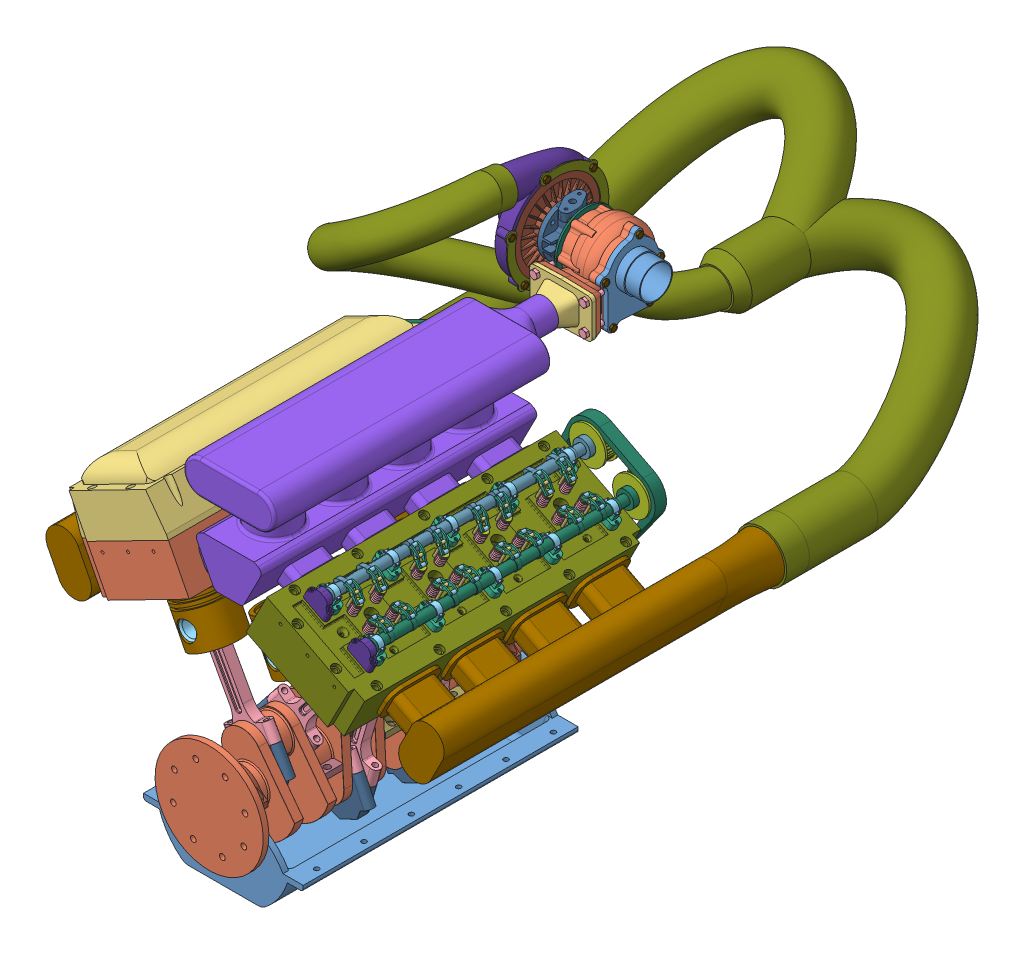
SolidWorks assembly ENSAMBLAJE DE MOTOR V8, configuration Predeterminado. Lengths in mm. (continued)
Mates (geometry in assembly coordinates): (continued)
- Concéntrica259: concentric: cylinder of CUBIERTA DE SOPORTE DE ARBOL DE LEVAS-22 through (209.4015 209.8469 383.5) axis (0.455744 0.890111 0) radius 1.25; cylinder of SOPORTE DE ARBOL DE LEVAS-22 through (208.0343 207.1766 383.5) axis (0.455744 0.890111 0) radius 1
- Concéntrica260: concentric: cylinder of CUBIERTA DE SOPORTE DE ARBOL DE LEVAS-22 through (209.4015 209.8469 389.5) axis (0.455744 0.890111 0) radius 1.25; cylinder of SOPORTE DE ARBOL DE LEVAS-22 through (208.0343 207.1766 389.5) axis (0.455744 0.890111 0) radius 1
- Concéntrica261: concentric: cylinder of assembly; cylinder of assembly; cylinder of CUBIERTA DE SOPORTE DE ARBOL DE LEVAS-23 through (121.6935 251.3837 391.5) axis (0 0 -1) radius 9.9624; cylinder of SOPORTE DE ARBOL DE LEVAS-23 through (121.6935 251.3837 391.5) axis (0 0 -1) radius 8.5
- Concéntrica262: concentric: cylinder of CUBIERTA DE SOPORTE DE ARBOL DE LEVAS-23 through (132.8519 249.0408 389.5) axis (0.455744 0.890111 0) radius 1.25; cylinder of SOPORTE DE ARBOL DE LEVAS-23 through (131.4847 246.3705 389.5) axis (0.455744 0.890111 0) radius 1
- Concéntrica263: concentric: cylinder of CUBIERTA DE SOPORTE DE ARBOL DE LEVAS-23 through (132.8519 249.0408 383.5) axis (0.455744 0.890111 0) radius 1.25; cylinder of SOPORTE DE ARBOL DE LEVAS-23 through (131.4847 246.3705 383.5) axis (0.455744 0.890111 0) radius 1
- Concéntrica264: concentric: cylinder of assembly; cylinder of assembly; cylinder of CUBIERTA DE SOPORTE DE ARBOL DE LEVAS-21 through (198.243 212.1897 288.5) axis (0 0 -1) radius 9.9624; cylinder of SOPORTE DE ARBOL DE LEVAS-21 through (198.243 212.1897 288.5) axis (0 0 -1) radius 8.5
- Concéntrica265: concentric: cylinder of CUBIERTA DE SOPORTE DE ARBOL DE LEVAS-21 through (209.4015 209.8469 286.5) axis (0.455744 0.890111 0) radius 1.25; cylinder of SOPORTE DE ARBOL DE LEVAS-21 through (208.0343 207.1766 286.5) axis (0.455744 0.890111 0) radius 1
- Concéntrica266: concentric: cylinder of CUBIERTA DE SOPORTE DE ARBOL DE LEVAS-21 through (209.4015 209.8469 280.5) axis (0.455744 0.890111 0) radius 1; cylinder of SOPORTE DE ARBOL DE LEVAS-21 through (208.0343 207.1766 280.5) axis (0.455744 0.890111 0) radius 1
- Paralelo12: parallel: cylinder of CUBIERTA DE SOPORTE DE ARBOL DE LEVAS-18 through (209.4015 209.8469 492.5) axis (0.455744 0.890111 0) radius 1.25; cylinder of SOPORTE DE ARBOL DE LEVAS-18 through (208.8175 195.541 489.5) axis (0.455744 0.890111 0) radius 2.5
- Concéntrica268: concentric: cylinder of CUBIERTA DE SOPORTE DE ARBOL DE LEVAS-18 through (209.4015 209.8469 486.5) axis (0.455744 0.890111 0) radius 1.25; circle of SOPORTE DE ARBOL DE LEVAS-18
- Concéntrica269: concentric: cylinder of CUBIERTA DE SOPORTE DE ARBOL DE LEVAS-18 through (198.243 212.1897 494.5) axis (0 0 -1) radius 9.9624; cylinder of SOPORTE DE ARBOL DE LEVAS-18 through (198.243 212.1897 494.5) axis (0 0 -1) radius 8.5
- Concéntrica270: concentric: cylinder of assembly; cylinder of assembly; cylinder of CUBIERTA DE SOPORTE DE ARBOL DE LEVAS-16 through (198.243 212.1897 597.5) axis (0 0 -1) radius 9.9624; cylinder of SOPORTE DE ARBOL DE LEVAS-16 through (198.243 212.1897 597.5) axis (0 0 -1) radius 8.5
- Concéntrica271: concentric: cylinder of CUBIERTA DE SOPORTE DE ARBOL DE LEVAS-16 through (189.8191 219.8733 595.5) axis (0.455744 0.890111 0) radius 1; cylinder of SOPORTE DE ARBOL DE LEVAS-16 through (188.4518 217.2029 595.5) axis (0.455744 0.890111 0) radius 1
- Concéntrica272: concentric: cylinder of CUBIERTA DE SOPORTE DE ARBOL DE LEVAS-16 through (189.8191 219.8733 589.5) axis (0.455744 0.890111 0) radius 1.25; cylinder of SOPORTE DE ARBOL DE LEVAS-16 through (188.4518 217.2029 589.5) axis (0.455744 0.890111 0) radius 1
- Concéntrica274: concentric: cylinder of assembly; cylinder of assembly; cylinder of CUBIERTA DE SOPORTE DE ARBOL DE LEVAS-20 through (121.6935 251.3837 597.5) axis (0 0 -1) radius 9.9624; cylinder of SOPORTE DE ARBOL DE LEVAS-20 through (121.6935 251.3837 597.5) axis (0 0 -1) radius 8.5
- Concéntrica275: concentric: cylinder of CUBIERTA DE SOPORTE DE ARBOL DE LEVAS-20 through (113.2695 259.0672 595.5) axis (0.455744 0.890111 0) radius 1.25; cylinder of SOPORTE DE ARBOL DE LEVAS-20 through (111.9023 256.3969 595.5) axis (0.455744 0.890111 0) radius 1
- Concéntrica276: concentric: cylinder of CUBIERTA DE SOPORTE DE ARBOL DE LEVAS-20 through (113.2695 259.0672 589.5) axis (0.455744 0.890111 0) radius 1.25; cylinder of SOPORTE DE ARBOL DE LEVAS-20 through (111.9023 256.3969 589.5) axis (0.455744 0.890111 0) radius 1
- Concéntrica277: concentric: cylinder of assembly; cylinder of assembly; cylinder of CUBIERTA DE SOPORTE DE ARBOL DE LEVAS-19 through (121.6935 251.3837 494.5) axis (0 0 -1) radius 9.9624; cylinder of SOPORTE DE ARBOL DE LEVAS-19 through (121.6935 251.3837 494.5) axis (0 0 -1) radius 8.5
- Concéntrica278: concentric: cylinder of CUBIERTA DE SOPORTE DE ARBOL DE LEVAS-19 through (113.2695 259.0672 492.5) axis (0.455744 0.890111 0) radius 1; cylinder of SOPORTE DE ARBOL DE LEVAS-19 through (111.9023 256.3969 492.5) axis (0.455744 0.890111 0) radius 1
- Concéntrica279: concentric: cylinder of CUBIERTA DE SOPORTE DE ARBOL DE LEVAS-19 through (113.2695 259.0672 486.5) axis (0.455744 0.890111 0) radius 1.25; cylinder of SOPORTE DE ARBOL DE LEVAS-19 through (111.9023 256.3969 486.5) axis (0.455744 0.890111 0) radius 1
- Concéntrica280: concentric: cylinder of assembly; cylinder of assembly; cylinder of CUBIERTA DE SOPORTE DE ARBOL DE LEVAS-15 through (-150.1483 251.4202 408.25) axis (0 0 -1) radius 9.9624; cylinder of SOPORTE DE ARBOL DE LEVAS-15 through (-150.1483 251.4202 408.25) axis (0 0 -1) radius 8.5
- Concéntrica281: concentric: cylinder of CUBIERTA DE SOPORTE DE ARBOL DE LEVAS-15 through (-161.3067 249.0773 400.25) axis (-0.455744 0.890111 0) radius 1; cylinder of SOPORTE DE ARBOL DE LEVAS-15 through (-159.9395 246.407 400.25) axis (-0.455744 0.890111 0) radius 1
- Concéntrica282: concentric: cylinder of CUBIERTA DE SOPORTE DE ARBOL DE LEVAS-15 through (-161.3067 249.0773 406.25) axis (-0.455744 0.890111 0) radius 1.25; cylinder of SOPORTE DE ARBOL DE LEVAS-15 through (-159.9395 246.407 406.25) axis (-0.455744 0.890111 0) radius 1
- Concéntrica283: concentric: cylinder of assembly; cylinder of assembly; cylinder of CUBIERTA DE SOPORTE DE ARBOL DE LEVAS-17 through (121.6935 251.3837 700.5) axis (0 0 -1) radius 9.9624; cylinder of SOPORTE DE ARBOL DE LEVAS-17 through (121.6935 251.3837 700.5) axis (0 0 -1) radius 8.5
- Concéntrica284: concentric: cylinder of CUBIERTA DE SOPORTE DE ARBOL DE LEVAS-17 through (113.2695 259.0672 698.5) axis (0.455744 0.890111 0) radius 1; cylinder of SOPORTE DE ARBOL DE LEVAS-17 through (111.9023 256.3969 698.5) axis (0.455744 0.890111 0) radius 1
- Concéntrica285: concentric: cylinder of CUBIERTA DE SOPORTE DE ARBOL DE LEVAS-17 through (113.2695 259.0672 692.5) axis (0.455744 0.890111 0) radius 1.25; cylinder of SOPORTE DE ARBOL DE LEVAS-17 through (111.9023 256.3969 692.5) axis (0.455744 0.890111 0) radius 1
- Coincidente129: coincident: plane of CULATA_IZQUIERDO-2 through (214.9378 178.9259 760.5) normal (0.455744 0.890111 0); plane of SOPORTE DE ARBOL DE LEVAS-16 through (173.0848 200.3549 592.5) normal (-0.455744 -0.890111 0)
- Concéntrica286: concentric: cylinder of CULATA_IZQUIERDO-2 through (203.3486 184.8597 592.5) axis (0.455744 0.890111 0) radius 1.7; cylinder of SOPORTE DE ARBOL DE LEVAS-16 through (208.8175 195.541 592.5) axis (0.455744 0.890111 0) radius 2.5
- Concéntrica287: concentric: cylinder of CULATA_IZQUIERDO-2 through (173.0848 200.3549 592.5) axis (0.455744 0.890111 0) radius 1.7; cylinder of SOPORTE DE ARBOL DE LEVAS-16 through (178.5537 211.0363 592.5) axis (0.455744 0.890111 0) radius 2.5
- Coincidente130: coincident: plane of CULATA_IZQUIERDO-2 through (214.9378 178.9259 760.5) normal (0.455744 0.890111 0); plane of SOPORTE DE ARBOL DE LEVAS-18 through (173.0848 200.3549 489.5) normal (-0.455744 -0.890111 0)
- Concéntrica288: concentric: cylinder of CULATA_IZQUIERDO-2 through (203.3486 184.8597 489.5) axis (0.455744 0.890111 0) radius 1.7; circle of SOPORTE DE ARBOL DE LEVAS-18
- Concéntrica289: concentric: cylinder of CULATA_IZQUIERDO-2 through (173.0848 200.3549 489.5) axis (0.455744 0.890111 0) radius 1.7; cylinder of SOPORTE DE ARBOL DE LEVAS-18 through (178.5537 211.0363 489.5) axis (0.455744 0.890111 0) radius 1.6
- Coincidente131: coincident: plane of CULATA_IZQUIERDO-2 through (214.9378 178.9259 760.5) normal (0.455744 0.890111 0); plane of SOPORTE DE ARBOL DE LEVAS-22 through (173.0848 200.3549 386.5) normal (-0.455744 -0.890111 0)
- Concéntrica290: concentric: cylinder of CULATA_IZQUIERDO-2 through (203.3486 184.8597 386.5) axis (0.455744 0.890111 0) radius 1.7; cylinder of SOPORTE DE ARBOL DE LEVAS-22 through (208.8175 195.541 386.5) axis (0.455744 0.890111 0) radius 1.6
- Concéntrica291: concentric: cylinder of CULATA_IZQUIERDO-2 through (173.0848 200.3549 386.5) axis (0.455744 0.890111 0) radius 1.7; cylinder of SOPORTE DE ARBOL DE LEVAS-22 through (178.5537 211.0363 386.5) axis (0.455744 0.890111 0) radius 1.6
- Coincidente132: coincident: plane of CULATA_IZQUIERDO-2 through (214.9378 178.9259 760.5) normal (0.455744 0.890111 0); plane of SOPORTE DE ARBOL DE LEVAS-21 through (173.0848 200.3549 283.5) normal (-0.455744 -0.890111 0)
- Concéntrica292: concentric: cylinder of CULATA_IZQUIERDO-2 through (203.3486 184.8597 283.5) axis (0.455744 0.890111 0) radius 1.7; cylinder of SOPORTE DE ARBOL DE LEVAS-21 through (208.8175 195.541 283.5) axis (0.455744 0.890111 0) radius 1.6
- Concéntrica293: concentric: cylinder of CULATA_IZQUIERDO-2 through (173.0848 200.3549 283.5) axis (0.455744 0.890111 0) radius 1.7; cylinder of SOPORTE DE ARBOL DE LEVAS-21 through (178.5537 211.0363 283.5) axis (0.455744 0.890111 0) radius 1.6
- Coincidente134: coincident: plane of CULATA_IZQUIERDO-2 through (214.9378 178.9259 760.5) normal (0.455744 0.890111 0); plane of SOPORTE DE ARBOL DE LEVAS-24 through (96.5352 239.5489 283.5) normal (-0.455744 -0.890111 0)
- Concéntrica294: concentric: cylinder of CULATA_IZQUIERDO-2 through (126.799 224.0536 283.5) axis (0.455744 0.890111 0) radius 1.7; circle of SOPORTE DE ARBOL DE LEVAS-24
- Concéntrica295: concentric: cylinder of CULATA_IZQUIERDO-2 through (96.5352 239.5489 283.5) axis (0.455744 0.890111 0) radius 1.7; cylinder of SOPORTE DE ARBOL DE LEVAS-24 through (102.0042 250.2302 283.5) axis (0.455744 0.890111 0) radius 1.6
- Coincidente135: coincident: plane of CULATA_IZQUIERDO-2 through (214.9378 178.9259 760.5) normal (0.455744 0.890111 0); plane of SOPORTE DE ARBOL DE LEVAS-23 through (96.5352 239.5489 386.5) normal (-0.455744 -0.890111 0)
- Concéntrica296: concentric: cylinder of CULATA_IZQUIERDO-2 through (126.799 224.0536 386.5) axis (0.455744 0.890111 0) radius 1.7; cylinder of SOPORTE DE ARBOL DE LEVAS-23 through (132.2679 234.7349 386.5) axis (0.455744 0.890111 0) radius 2.5
- Concéntrica297: concentric: cylinder of CULATA_IZQUIERDO-2 through (96.5352 239.5489 386.5) axis (0.455744 0.890111 0) radius 1.7; cylinder of SOPORTE DE ARBOL DE LEVAS-23 through (102.0042 250.2302 386.5) axis (0.455744 0.890111 0) radius 1.6
- Coincidente136: coincident: plane of CULATA_IZQUIERDO-2 through (214.9378 178.9259 760.5) normal (0.455744 0.890111 0); plane of SOPORTE DE ARBOL DE LEVAS-19 through (96.5352 239.5489 489.5) normal (-0.455744 -0.890111 0)
- Concéntrica298: concentric: cylinder of CULATA_IZQUIERDO-2 through (126.799 224.0536 489.5) axis (0.455744 0.890111 0) radius 1.7; cylinder of SOPORTE DE ARBOL DE LEVAS-19 through (132.2679 234.7349 489.5) axis (0.455744 0.890111 0) radius 2.5
- Concéntrica299: concentric: cylinder of CULATA_IZQUIERDO-2 through (96.5352 239.5489 489.5) axis (0.455744 0.890111 0) radius 1.7; cylinder of SOPORTE DE ARBOL DE LEVAS-19 through (102.0042 250.2302 489.5) axis (0.455744 0.890111 0) radius 1.6
- Coincidente137: coincident: plane of CULATA_IZQUIERDO-2 through (214.9378 178.9259 760.5) normal (0.455744 0.890111 0); plane of SOPORTE DE ARBOL DE LEVAS-20 through (96.5352 239.5489 592.5) normal (-0.455744 -0.890111 0)
- Concéntrica300: concentric: cylinder of CULATA_IZQUIERDO-2 through (126.799 224.0536 592.5) axis (0.455744 0.890111 0) radius 1.7; cylinder of SOPORTE DE ARBOL DE LEVAS-20 through (132.2679 234.7349 592.5) axis (0.455744 0.890111 0) radius 2.5
- Concéntrica301: concentric: cylinder of CULATA_IZQUIERDO-2 through (96.5352 239.5489 592.5) axis (0.455744 0.890111 0) radius 1.7; circle of SOPORTE DE ARBOL DE LEVAS-20
- Coincidente138: coincident: plane of CULATA_IZQUIERDO-2 through (214.9378 178.9259 760.5) normal (0.455744 0.890111 0); plane of SOPORTE DE ARBOL DE LEVAS-17 through (96.5352 239.5489 695.5) normal (-0.455744 -0.890111 0)
- Concéntrica302: concentric: cylinder of CULATA_IZQUIERDO-2 through (126.799 224.0536 695.5) axis (0.455744 0.890111 0) radius 1.7; cylinder of SOPORTE DE ARBOL DE LEVAS-17 through (132.2679 234.7349 695.5) axis (0.455744 0.890111 0) radius 2.5
- Concéntrica303: concentric: cylinder of CULATA_IZQUIERDO-2 through (96.5352 239.5489 695.5) axis (0.455744 0.890111 0) radius 1.7; cylinder of SOPORTE DE ARBOL DE LEVAS-17 through (102.0042 250.2302 695.5) axis (0.455744 0.890111 0) radius 1.6
- Coincidente139: coincident: plane of ARBOL DE LEVAS DE ADMISIÓN_IZQUIERDO-2 through (121.6935 251.3837 278.5) normal (0 0 1); plane of SOPORTE DE ARBOL DE LEVAS-24 through (96.5352 239.5489 278.5) normal (0 0 -1)
- Concéntrica363: concentric: cylinder of assembly; cylinder of assembly; cylinder of ARBOL DE LEVAS DE ADMISIÓN_DERECHO-1 through (-150.1483 251.4202 733.25) axis (0 0 -1) radius 8.5; cylinder of SOPORTE EXTERNO DE ARBOL DE LEVAS-4 through (-150.1483 251.4202 734.25) axis (0 0 -1) radius 8.5
- Concéntrica356: concentric: cylinder of ARBOL DE LEVAS DE ESCAPE_DERECHO-1 through (-226.6978 212.2262 733.25) axis (0 0 -1) radius 8.5; cylinder of SOPORTE EXTERNO DE ARBOL DE LEVAS-3 through (-226.6978 212.2262 734.25) axis (0 0 -1) radius 8.5
- Concéntrica306: concentric: cylinder of assembly; cylinder of assembly; cylinder of CUBIERTA DE SOPORTE DE ARBOL DE LEVAS-30 through (-150.1483 251.4202 515.25) axis (0 0 -1) radius 9.9624; cylinder of SOPORTE DE ARBOL DE LEVAS-30 through (-150.1483 251.4202 515.25) axis (0 0 -1) radius 8.5
- Concéntrica307: concentric: cylinder of CUBIERTA DE SOPORTE DE ARBOL DE LEVAS-30 through (-161.3067 249.0773 513.25) axis (-0.455744 0.890111 0) radius 1.25; cylinder of SOPORTE DE ARBOL DE LEVAS-30 through (-159.9395 246.407 513.25) axis (-0.455744 0.890111 0) radius 1
- Concéntrica308: concentric: cylinder of CUBIERTA DE SOPORTE DE ARBOL DE LEVAS-30 through (-161.3067 249.0773 507.25) axis (-0.455744 0.890111 0) radius 1.25; cylinder of SOPORTE DE ARBOL DE LEVAS-30 through (-159.9395 246.407 507.25) axis (-0.455744 0.890111 0) radius 1
- Concéntrica309: concentric: cylinder of assembly; cylinder of assembly; cylinder of CUBIERTA DE SOPORTE DE ARBOL DE LEVAS-28 through (-226.6978 212.2262 515.25) axis (0 0 -1) radius 9.9624; cylinder of SOPORTE DE ARBOL DE LEVAS-28 through (-226.6978 212.2262 515.25) axis (0 0 -1) radius 8.5
- Concéntrica310: concentric: cylinder of CUBIERTA DE SOPORTE DE ARBOL DE LEVAS-28 through (-237.8563 209.8834 507.25) axis (-0.455744 0.890111 0) radius 1.25; cylinder of SOPORTE DE ARBOL DE LEVAS-28 through (-236.489 207.213 507.25) axis (-0.455744 0.890111 0) radius 1
- Concéntrica311: concentric: cylinder of CUBIERTA DE SOPORTE DE ARBOL DE LEVAS-28 through (-218.2738 219.9097 507.25) axis (-0.455744 0.890111 0) radius 1.25; cylinder of SOPORTE DE ARBOL DE LEVAS-28 through (-216.9066 217.2394 507.25) axis (-0.455744 0.890111 0) radius 1
- Concéntrica312: concentric: cylinder of assembly; cylinder of assembly; cylinder of CUBIERTA DE SOPORTE DE ARBOL DE LEVAS-29 through (-226.6978 212.2262 721.25) axis (0 0 -1) radius 9.9624; cylinder of SOPORTE DE ARBOL DE LEVAS-29 through (-226.6978 212.2262 721.25) axis (0 0 -1) radius 8.5
- Concéntrica313: concentric: cylinder of CUBIERTA DE SOPORTE DE ARBOL DE LEVAS-29 through (-237.8563 209.8834 713.25) axis (-0.455744 0.890111 0) radius 1.25; cylinder of SOPORTE DE ARBOL DE LEVAS-29 through (-236.489 207.213 713.25) axis (-0.455744 0.890111 0) radius 1
- Concéntrica314: concentric: cylinder of CUBIERTA DE SOPORTE DE ARBOL DE LEVAS-29 through (-237.8563 209.8834 719.25) axis (-0.455744 0.890111 0) radius 1.25; cylinder of SOPORTE DE ARBOL DE LEVAS-29 through (-236.489 207.213 719.25) axis (-0.455744 0.890111 0) radius 1
- Concéntrica315: concentric: cylinder of assembly; cylinder of assembly; cylinder of CUBIERTA DE SOPORTE DE ARBOL DE LEVAS-32 through (-226.6978 212.2262 301.25) axis (0 0 -1) radius 9.9624; cylinder of SOPORTE DE ARBOL DE LEVAS-32 through (-226.6978 212.2262 301.25) axis (0 0 -1) radius 8.5
- Concéntrica316: concentric: cylinder of CUBIERTA DE SOPORTE DE ARBOL DE LEVAS-32 through (-237.8563 209.8834 299.25) axis (-0.455744 0.890111 0) radius 1.25; cylinder of SOPORTE DE ARBOL DE LEVAS-32 through (-236.489 207.213 299.25) axis (-0.455744 0.890111 0) radius 1
- Concéntrica317: concentric: cylinder of CUBIERTA DE SOPORTE DE ARBOL DE LEVAS-32 through (-237.8563 209.8834 293.25) axis (-0.455744 0.890111 0) radius 1.25; cylinder of SOPORTE DE ARBOL DE LEVAS-32 through (-236.489 207.213 293.25) axis (-0.455744 0.890111 0) radius 1
- Concéntrica318: concentric: cylinder of assembly; cylinder of assembly; cylinder of CUBIERTA DE SOPORTE DE ARBOL DE LEVAS-33 through (-226.6978 212.2262 408.25) axis (0 0 -1) radius 9.9624; cylinder of SOPORTE DE ARBOL DE LEVAS-33 through (-226.6978 212.2262 408.25) axis (0 0 -1) radius 8.5
- Concéntrica319: concentric: cylinder of CUBIERTA DE SOPORTE DE ARBOL DE LEVAS-33 through (-237.8563 209.8834 406.25) axis (-0.455744 0.890111 0) radius 1.25; circle of SOPORTE DE ARBOL DE LEVAS-33
- Concéntrica320: concentric: cylinder of CUBIERTA DE SOPORTE DE ARBOL DE LEVAS-33 through (-237.8563 209.8834 400.25) axis (-0.455744 0.890111 0) radius 1.25; cylinder of SOPORTE DE ARBOL DE LEVAS-33 through (-236.489 207.213 400.25) axis (-0.455744 0.890111 0) radius 1
- Concéntrica321: concentric: cylinder of assembly; cylinder of assembly; cylinder of SOPORTE DE ARBOL DE LEVAS-26 through (-226.6978 212.2262 622.25) axis (0 0 -1) radius 8.5; cylinder of CUBIERTA DE SOPORTE DE ARBOL DE LEVAS-27 through (-226.6978 212.2262 622.25) axis (0 0 -1) radius 9.9624
- Concéntrica322: concentric: cylinder of SOPORTE DE ARBOL DE LEVAS-26 through (-236.489 207.213 614.25) axis (-0.455744 0.890111 0) radius 1; cylinder of CUBIERTA DE SOPORTE DE ARBOL DE LEVAS-27 through (-237.8563 209.8834 614.25) axis (-0.455744 0.890111 0) radius 1.25
- Concéntrica323: concentric: cylinder of SOPORTE DE ARBOL DE LEVAS-26 through (-236.489 207.213 620.25) axis (-0.455744 0.890111 0) radius 1; cylinder of CUBIERTA DE SOPORTE DE ARBOL DE LEVAS-27 through (-237.8563 209.8834 620.25) axis (-0.455744 0.890111 0) radius 1.25
- Concéntrica324: concentric: cylinder of assembly; cylinder of assembly; cylinder of SOPORTE DE ARBOL DE LEVAS-27 through (-150.1483 251.4202 721.25) axis (0 0 -1) radius 8.5; cylinder of CUBIERTA DE SOPORTE DE ARBOL DE LEVAS-31 through (-150.1483 251.4202 721.25) axis (0 0 -1) radius 9.9624
- Concéntrica325: concentric: cylinder of SOPORTE DE ARBOL DE LEVAS-27 through (-159.9395 246.407 713.25) axis (-0.455744 0.890111 0) radius 1; cylinder of CUBIERTA DE SOPORTE DE ARBOL DE LEVAS-31 through (-161.3067 249.0773 713.25) axis (-0.455744 0.890111 0) radius 1.25
- Concéntrica326: concentric: cylinder of SOPORTE DE ARBOL DE LEVAS-27 through (-159.9395 246.407 719.25) axis (-0.455744 0.890111 0) radius 1; cylinder of CUBIERTA DE SOPORTE DE ARBOL DE LEVAS-31 through (-161.3067 249.0773 719.25) axis (-0.455744 0.890111 0) radius 1.25
- Concéntrica327: concentric: cylinder of assembly; cylinder of assembly; cylinder of CUBIERTA DE SOPORTE DE ARBOL DE LEVAS-25 through (-150.1483 251.4202 622.25) axis (0 0 -1) radius 9.9624; cylinder of SOPORTE DE ARBOL DE LEVAS-25 through (-150.1483 251.4202 622.25) axis (0 0 -1) radius 8.5
- Concéntrica328: concentric: cylinder of CUBIERTA DE SOPORTE DE ARBOL DE LEVAS-25 through (-161.3067 249.0773 620.25) axis (-0.455744 0.890111 0) radius 1.25; cylinder of SOPORTE DE ARBOL DE LEVAS-25 through (-159.9395 246.407 620.25) axis (-0.455744 0.890111 0) radius 1
- Concéntrica329: concentric: cylinder of CUBIERTA DE SOPORTE DE ARBOL DE LEVAS-25 through (-161.3067 249.0773 614.25) axis (-0.455744 0.890111 0) radius 1.25; cylinder of SOPORTE DE ARBOL DE LEVAS-25 through (-159.9395 246.407 614.25) axis (-0.455744 0.890111 0) radius 1
- Concéntrica330: concentric: cylinder of assembly; cylinder of assembly; cylinder of CUBIERTA DE SOPORTE DE ARBOL DE LEVAS-26 through (-150.1483 251.4202 301.25) axis (0 0 -1) radius 9.9624; cylinder of SOPORTE DE ARBOL DE LEVAS-31 through (-150.1483 251.4202 301.25) axis (0 0 -1) radius 8.5
- Concéntrica331: concentric: cylinder of CUBIERTA DE SOPORTE DE ARBOL DE LEVAS-26 through (-141.7243 259.1037 293.25) axis (-0.455744 0.890111 0) radius 1.25; cylinder of SOPORTE DE ARBOL DE LEVAS-31 through (-140.357 256.4333 293.25) axis (-0.455744 0.890111 0) radius 1
- Concéntrica332: concentric: cylinder of CUBIERTA DE SOPORTE DE ARBOL DE LEVAS-26 through (-161.3067 249.0773 299.25) axis (-0.455744 0.890111 0) radius 1.25; cylinder of SOPORTE DE ARBOL DE LEVAS-31 through (-159.9395 246.407 299.25) axis (-0.455744 0.890111 0) radius 1
- Coincidente141: coincident: plane of CULATA_DERECHO-1 through (-100.6544 252.0454 253.5) normal (-0.455744 0.890111 0); plane of SOPORTE DE ARBOL DE LEVAS-29 through (-231.8033 184.8961 716.25) normal (0.455744 -0.890111 0)
- Concéntrica333: concentric: cylinder of CULATA_DERECHO-1 through (-231.8033 184.8961 716.25) axis (-0.455744 0.890111 0) radius 1.7; cylinder of SOPORTE DE ARBOL DE LEVAS-29 through (-237.2723 195.5775 716.25) axis (-0.455744 0.890111 0) radius 2.5
- Concéntrica334: concentric: cylinder of CULATA_DERECHO-1 through (-201.5396 200.3914 716.25) axis (-0.455744 0.890111 0) radius 1.7; cylinder of SOPORTE DE ARBOL DE LEVAS-29 through (-207.0085 211.0727 716.25) axis (-0.455744 0.890111 0) radius 1.6
- Coincidente142: coincident: plane of CULATA_DERECHO-1 through (-100.6544 252.0454 253.5) normal (-0.455744 0.890111 0); plane of SOPORTE DE ARBOL DE LEVAS-27 through (-155.2538 224.0901 716.25) normal (0.455744 -0.890111 0)
- Concéntrica336: concentric: cylinder of CULATA_DERECHO-1 through (-155.2538 224.0901 716.25) axis (-0.455744 0.890111 0) radius 1.7; cylinder of SOPORTE DE ARBOL DE LEVAS-27 through (-160.7227 234.7714 716.25) axis (-0.455744 0.890111 0) radius 2.5
- Concéntrica337: concentric: cylinder of CULATA_DERECHO-1 through (-124.99 239.5854 716.25) axis (-0.455744 0.890111 0) radius 1.7; cylinder of SOPORTE DE ARBOL DE LEVAS-27 through (-130.4589 250.2667 716.25) axis (-0.455744 0.890111 0) radius 1.6
- Coincidente143: coincident: plane of CULATA_DERECHO-1 through (-100.6544 252.0454 253.5) normal (-0.455744 0.890111 0); plane of SOPORTE DE ARBOL DE LEVAS-26 through (-231.8033 184.8961 617.25) normal (0.455744 -0.890111 0)
- Concéntrica338: concentric: cylinder of CULATA_DERECHO-1 through (-231.8033 184.8961 617.25) axis (-0.455744 0.890111 0) radius 1.7; cylinder of SOPORTE DE ARBOL DE LEVAS-26 through (-237.2723 195.5775 617.25) axis (-0.455744 0.890111 0) radius 2.5
- Concéntrica339: concentric: cylinder of CULATA_DERECHO-1 through (-201.5396 200.3914 617.25) axis (-0.455744 0.890111 0) radius 1.7; cylinder of SOPORTE DE ARBOL DE LEVAS-26 through (-207.0085 211.0727 617.25) axis (-0.455744 0.890111 0) radius 1.6
- Coincidente144: coincident: plane of CULATA_DERECHO-1 through (-100.6544 252.0454 253.5) normal (-0.455744 0.890111 0); plane of SOPORTE DE ARBOL DE LEVAS-28 through (-231.8033 184.8961 510.25) normal (0.455744 -0.890111 0)
- Concéntrica340: concentric: cylinder of CULATA_DERECHO-1 through (-231.8033 184.8961 510.25) axis (-0.455744 0.890111 0) radius 1.7; cylinder of SOPORTE DE ARBOL DE LEVAS-28 through (-237.2723 195.5775 510.25) axis (-0.455744 0.890111 0) radius 2.5
- Concéntrica341: concentric: cylinder of CULATA_DERECHO-1 through (-201.5396 200.3914 510.25) axis (-0.455744 0.890111 0) radius 1.7; cylinder of SOPORTE DE ARBOL DE LEVAS-28 through (-207.0085 211.0727 510.25) axis (-0.455744 0.890111 0) radius 1.6
- Coincidente145: coincident: plane of CULATA_DERECHO-1 through (-100.6544 252.0454 253.5) normal (-0.455744 0.890111 0); plane of SOPORTE DE ARBOL DE LEVAS-30 through (-155.2538 224.0901 510.25) normal (0.455744 -0.890111 0)
- Concéntrica342: concentric: cylinder of CULATA_DERECHO-1 through (-155.2538 224.0901 510.25) axis (-0.455744 0.890111 0) radius 1.7; cylinder of SOPORTE DE ARBOL DE LEVAS-30 through (-160.7227 234.7714 510.25) axis (-0.455744 0.890111 0) radius 2.5
- Concéntrica343: concentric: cylinder of CULATA_DERECHO-1 through (-124.99 239.5854 510.25) axis (-0.455744 0.890111 0) radius 1.7; cylinder of SOPORTE DE ARBOL DE LEVAS-30 through (-130.4589 250.2667 510.25) axis (-0.455744 0.890111 0) radius 1.6
- Coincidente146: coincident: plane of CULATA_DERECHO-1 through (-100.6544 252.0454 253.5) normal (-0.455744 0.890111 0); plane of SOPORTE DE ARBOL DE LEVAS-33 through (-231.8033 184.8961 403.25) normal (0.455744 -0.890111 0)
- Concéntrica344: concentric: cylinder of CULATA_DERECHO-1 through (-231.8033 184.8961 403.25) axis (-0.455744 0.890111 0) radius 1.7; cylinder of SOPORTE DE ARBOL DE LEVAS-33 through (-237.2723 195.5775 403.25) axis (-0.455744 0.890111 0) radius 2.5
- Concéntrica345: concentric: cylinder of CULATA_DERECHO-1 through (-201.5396 200.3914 403.25) axis (-0.455744 0.890111 0) radius 1.7; cylinder of SOPORTE DE ARBOL DE LEVAS-33 through (-207.0085 211.0727 403.25) axis (-0.455744 0.890111 0) radius 1.6
- Coincidente147: coincident: plane of CULATA_DERECHO-1 through (-100.6544 252.0454 253.5) normal (-0.455744 0.890111 0); plane of SOPORTE DE ARBOL DE LEVAS-32 through (-231.8033 184.8961 296.25) normal (0.455744 -0.890111 0)
- Concéntrica346: concentric: cylinder of CULATA_DERECHO-1 through (-231.8033 184.8961 296.25) axis (-0.455744 0.890111 0) radius 1.7; cylinder of SOPORTE DE ARBOL DE LEVAS-32 through (-237.2723 195.5775 296.25) axis (-0.455744 0.890111 0) radius 1.6
- Concéntrica347: concentric: cylinder of CULATA_DERECHO-1 through (-201.5396 200.3914 296.25) axis (-0.455744 0.890111 0) radius 1.7; cylinder of SOPORTE DE ARBOL DE LEVAS-32 through (-207.0085 211.0727 296.25) axis (-0.455744 0.890111 0) radius 1.6
- Coincidente148: coincident: plane of CULATA_DERECHO-1 through (-100.6544 252.0454 253.5) normal (-0.455744 0.890111 0); plane of SOPORTE DE ARBOL DE LEVAS-31 through (-155.2538 224.0901 296.25) normal (0.455744 -0.890111 0)
- Concéntrica348: concentric: cylinder of CULATA_DERECHO-1 through (-155.2538 224.0901 296.25) axis (-0.455744 0.890111 0) radius 1.7; cylinder of SOPORTE DE ARBOL DE LEVAS-31 through (-160.7227 234.7714 296.25) axis (-0.455744 0.890111 0) radius 2.5
- Concéntrica349: concentric: cylinder of CULATA_DERECHO-1 through (-124.99 239.5854 296.25) axis (-0.455744 0.890111 0) radius 1.7; cylinder of SOPORTE DE ARBOL DE LEVAS-31 through (-130.4589 250.2667 296.25) axis (-0.455744 0.890111 0) radius 1.6
- Coincidente149: coincident: plane of CULATA_DERECHO-1 through (-100.6544 252.0454 253.5) normal (-0.455744 0.890111 0); plane of SOPORTE DE ARBOL DE LEVAS-15 through (-155.2538 224.0901 403.25) normal (0.455744 -0.890111 0)
- Concéntrica350: concentric: cylinder of CULATA_DERECHO-1 through (-155.2538 224.0901 403.25) axis (-0.455744 0.890111 0) radius 1.7; cylinder of SOPORTE DE ARBOL DE LEVAS-15 through (-160.7227 234.7714 403.25) axis (-0.455744 0.890111 0) radius 2.5
- Concéntrica351: concentric: cylinder of CULATA_DERECHO-1 through (-124.99 239.5854 403.25) axis (-0.455744 0.890111 0) radius 1.7; cylinder of SOPORTE DE ARBOL DE LEVAS-15 through (-130.4589 250.2667 403.25) axis (-0.455744 0.890111 0) radius 1.6
- Coincidente150: coincident: plane of CULATA_DERECHO-1 through (-100.6544 252.0454 253.5) normal (-0.455744 0.890111 0); plane of SOPORTE DE ARBOL DE LEVAS-25 through (-155.2538 224.0901 617.25) normal (0.455744 -0.890111 0)
- Concéntrica352: concentric: cylinder of CULATA_DERECHO-1 through (-155.2538 224.0901 617.25) axis (-0.455744 0.890111 0) radius 1.7; cylinder of SOPORTE DE ARBOL DE LEVAS-25 through (-160.7227 234.7714 617.25) axis (-0.455744 0.890111 0) radius 2.5
- Concéntrica353: concentric: cylinder of CULATA_DERECHO-1 through (-124.99 239.5854 617.25) axis (-0.455744 0.890111 0) radius 1.7; cylinder of SOPORTE DE ARBOL DE LEVAS-25 through (-130.4589 250.2667 617.25) axis (-0.455744 0.890111 0) radius 1.6
- Coincidente152: coincident: plane of ARBOL DE LEVAS DE ESCAPE_DERECHO-1 through (-226.6978 212.2262 721.25) normal (0 0 -1); plane of SOPORTE DE ARBOL DE LEVAS-29 through (-231.8033 184.8961 721.25) normal (0 0 1)
- Concéntrica360: concentric: cylinder of CULATA_DERECHO-1 through (-200.6495 200.8471 696.25) axis (-0.455744 0.890111 0) radius 2.25; cylinder of EJE DE CONTROL DE VÁLVULAS-9 through (-193.8133 187.4955 696.25) axis (0.455744 -0.890111 0) radius 2.25
- Coincidente153: coincident: circle of CULATA_DERECHO-1; plane of EJE DE CONTROL DE VÁLVULAS-9 through (-193.8133 187.4955 698.5) normal (0.455744 -0.890111 0)
- Tangente15: tangent: cylinder of SEGUIDOR DE LEVA-25 through (-201.8109 228.7811 692.45) axis (0 0 1) radius 3; plane of VÁLVULA-9 through (-201.9541 225.3374 696.25) normal (-0.455744 0.890111 0)
- Relación de posición de Leva Tangente11: cam tangent: cylinder of ARBOL DE LEVAS DE ESCAPE_DERECHO-1 through (-226.6978 212.2262 692.45) axis (0 0 1) radius 9; cylinder of SEGUIDOR DE LEVA-34 through (-228.9095 224.0206 692.45) axis (0 0 1) radius 3
- Paralelo16: parallel: plane of CULATA_DERECHO-1 through (-243.3926 178.9623 760.5) normal (0 0 1); plane of SOPORTE DE SEGUIDOR DE VÁLVULA-9 through (-210.1649 237.0305 703.05) normal (0 0 1)
- Coincidente154: coincident: plane of ARBOL DE LEVAS DE ADMISIÓN_DERECHO-1 through (-150.1483 251.4202 721.25) normal (0 0 -1); plane of SOPORTE DE ARBOL DE LEVAS-27 through (-155.2538 224.0901 721.25) normal (0 0 1)
- Relación de posición de engranaje2: gear = 1 : 2 mm: cylinder of assembly; cylinder of assembly; cylinder of CIGUEÑAL-1 through (-14.263 -103.8973 775.5) axis (0 0 -1) radius 94.8; cylinder of ARBOL DE LEVAS DE ADMISIÓN_DERECHO-1 through (-150.1483 251.4202 153.25) axis (0 0 -1) radius 8.5
- Concéntrica364: concentric: cylinder of assembly; cylinder of assembly; cylinder of CIGUEÑAL-1 through (-14.263 -103.8973 221.5) axis (0 0 1) radius 7.625; cylinder of ENGRANE CIGUEÑAL-1 through (-14.263 -103.8973 275) axis (0 0 -1) radius 7.625
- Concéntrica365: concentric: cylinder of ARBOL DE LEVAS DE ESCAPE_IZQUIERDO-2 through (198.243 212.1897 140.5) axis (0 0 -1) radius 8.5; cylinder of ENGRANE ARBOL DE LEVAS-1 through (198.243 212.1897 199) axis (0 0 1) radius 8.5
- Coincidente156: coincident: plane of ARBOL DE LEVAS DE ESCAPE_IZQUIERDO-2 through (187.5653 216.9587 208.5) normal (-0.628385 -0.777902 0); plane of ENGRANE ARBOL DE LEVAS-1 through (187.5653 216.9587 199) normal (0.628385 0.777902 0)
- Coincidente157: coincident: plane of ARBOL DE LEVAS DE ESCAPE_IZQUIERDO-2 through (198.243 212.1897 248.5) normal (0 0 -1); plane of ENGRANE ARBOL DE LEVAS-1 through (198.243 212.1897 248.5) normal (0 0 1)
- Concéntrica366: concentric: cylinder of ARBOL DE LEVAS DE ADMISIÓN_IZQUIERDO-2 through (121.6935 251.3837 140.5) axis (0 0 -1) radius 8.5; cylinder of ENGRANE ARBOL DE LEVAS-2 through (121.6935 251.3837 199) axis (0 0 1) radius 8.5
- Coincidente158: coincident: plane of ARBOL DE LEVAS DE ADMISIÓN_IZQUIERDO-2 through (111.7007 257.4583 208.5) normal (0.282857 0.959162 0); plane of ENGRANE ARBOL DE LEVAS-2 through (114.9139 256.5107 199) normal (-0.282857 -0.959162 0)
- Coincidente159: coincident: plane of ARBOL DE LEVAS DE ADMISIÓN_IZQUIERDO-2 through (121.6935 251.3837 248.5) normal (0 0 -1); plane of ENGRANE ARBOL DE LEVAS-2 through (121.6935 251.3837 248.5) normal (0 0 1)
- Coincidente160: coincident: plane of assembly; plane of assembly; plane of ARBOL DE LEVAS DE ADMISIÓN_DERECHO-1 through (-155.985 245.2409 208.5) normal (0.43783 -0.899058 0); plane of ENGRANE ARBOL DE LEVAS-3 through (-158.9968 243.7742 199) normal (-0.43783 0.899058 0)
- Concéntrica367: concentric: cylinder of ARBOL DE LEVAS DE ADMISIÓN_DERECHO-1 through (-150.1483 251.4202 153.25) axis (0 0 -1) radius 8.5; cylinder of ENGRANE ARBOL DE LEVAS-3 through (-150.1483 251.4202 199) axis (0 0 1) radius 8.5
- Coincidente161: coincident: plane of ARBOL DE LEVAS DE ADMISIÓN_DERECHO-1 through (-150.1483 251.4202 248.5) normal (0 0 -1); plane of ENGRANE ARBOL DE LEVAS-3 through (-150.1483 251.4202 248.5) normal (0 0 1)
- Coincidente162: coincident: plane of CIGUEÑAL-1 through (-14.1038 -111.5207 221.5) normal (-0.937671 -0.347525 0); plane of ENGRANE CIGUEÑAL-1 through (-14.1038 -111.5207 275) normal (0.937671 0.347525 0)
- Coincidente163: coincident: plane of CIGUEÑAL-1 through (-14.263 -103.8973 248.5) normal (0 0 -1); plane of ENGRANE CIGUEÑAL-1 through (-14.263 -103.8973 248.5) normal (0 0 1)
- Coincidente164: coincident: plane of ARBOL DE LEVAS DE ESCAPE_DERECHO-1 through (-237.9107 215.5472 208.5) normal (0.028509 0.999594 0); plane of ENGRANE ARBOL DE LEVAS-4 through (-234.562 215.4517 199) normal (-0.028509 -0.999594 0)
- Concéntrica368: concentric: cylinder of ARBOL DE LEVAS DE ESCAPE_DERECHO-1 through (-226.6978 212.2262 153.25) axis (0 0 -1) radius 8.5; cylinder of ENGRANE ARBOL DE LEVAS-4 through (-226.6978 212.2262 199) axis (0 0 1) radius 8.5
- Coincidente165: coincident: plane of ARBOL DE LEVAS DE ESCAPE_DERECHO-1 through (-226.6978 212.2262 248.5) normal (0 0 -1); plane of ENGRANE ARBOL DE LEVAS-4 through (-226.6978 212.2262 248.5) normal (0 0 1)
- Concéntrica369: concentric: cylinder of ARBOL DE LEVAS DE ESCAPE_IZQUIERDO-2 through (198.243 212.1897 221.5) axis (0 0 -1) radius 3.8; cylinder of TORNILLO CABEZA HEXAGONAL_ENGRANE DE ARBOL DE LEVAS-1 through (198.243 212.1897 271.5) axis (0 0 -1) radius 3.8
- Coincidente166: coincident: plane of ENGRANE ARBOL DE LEVAS-1 through (198.243 212.1897 221.5) normal (0 0 -1); plane of TORNILLO CABEZA HEXAGONAL_ENGRANE DE ARBOL DE LEVAS-1 through (198.243 212.1897 221.5) normal (0 0 1)
- Concéntrica370: concentric: cylinder of ARBOL DE LEVAS DE ADMISIÓN_IZQUIERDO-2 through (121.6935 251.3837 221.5) axis (0 0 -1) radius 3.8; cylinder of TORNILLO CABEZA HEXAGONAL_ENGRANE DE ARBOL DE LEVAS-2 through (121.6935 251.3837 271.5) axis (0 0 -1) radius 3.8
- Coincidente168: coincident: plane of ENGRANE ARBOL DE LEVAS-2 through (121.6935 251.3837 221.5) normal (0 0 -1); plane of TORNILLO CABEZA HEXAGONAL_ENGRANE DE ARBOL DE LEVAS-2 through (121.6935 251.3837 221.5) normal (0 0 1)
- Concéntrica371: concentric: cylinder of assembly; cylinder of assembly; cylinder of ARBOL DE LEVAS DE ADMISIÓN_DERECHO-1 through (-150.1483 251.4202 221.5) axis (0 0 -1) radius 3.8; cylinder of TORNILLO CABEZA HEXAGONAL_ENGRANE DE ARBOL DE LEVAS-4 through (-150.1483 251.4202 271.5) axis (0 0 -1) radius 3.8
- Coincidente169: coincident: plane of ENGRANE ARBOL DE LEVAS-3 through (-150.1483 251.4202 221.5) normal (0 0 -1); plane of TORNILLO CABEZA HEXAGONAL_ENGRANE DE ARBOL DE LEVAS-4 through (-150.1483 251.4202 221.5) normal (0 0 1)
- Concéntrica372: concentric: cylinder of ARBOL DE LEVAS DE ESCAPE_DERECHO-1 through (-226.6978 212.2262 221.5) axis (0 0 -1) radius 3.8; cylinder of TORNILLO CABEZA HEXAGONAL_ENGRANE DE ARBOL DE LEVAS-3 through (-226.6978 212.2262 271.5) axis (0 0 -1) radius 3.8
- Coincidente170: coincident: plane of ENGRANE ARBOL DE LEVAS-4 through (-226.6978 212.2262 221.5) normal (0 0 -1); plane of TORNILLO CABEZA HEXAGONAL_ENGRANE DE ARBOL DE LEVAS-3 through (-226.6978 212.2262 221.5) normal (0 0 1)
- Concéntrica377: concentric: cylinder of assembly; cylinder of assembly; cylinder of CIGUEÑAL-1 through (-14.263 -103.8973 221.5) axis (0 0 -1) radius 3.3; cylinder of TORNILLO CABEZA HEXAGONAL_ENGRANE DE ARBOL DE CIGÜEÑAL-1 through (-14.263 -103.8973 251.5) axis (0 0 -1) radius 3.3
- Coincidente171: coincident: plane of ENGRANE CIGUEÑAL-1 through (-14.263 -103.8973 221.5) normal (0 0 -1); plane of TORNILLO CABEZA HEXAGONAL_ENGRANE DE ARBOL DE CIGÜEÑAL-1 through (-14.263 -103.8973 221.5) normal (0 0 1)
- Concéntrica378: concentric: cylinder of ? through (-35.9136 133.3016 253.5) axis (0 0 -1) radius 4.5; cylinder of SOPORTE DE RODAMIENTO PARA LA BANDA-1 through (-35.9136 133.3016 248.5) axis (0 0 -1) radius 9
- Concéntrica379: concentric: cylinder of ? through (7.3876 108.3016 253.5) axis (0 0 -1) radius 4.5; cylinder of SOPORTE DE RODAMIENTO PARA LA BANDA-1 through (7.3876 108.3016 248.5) axis (0 0 -1) radius 9
- Concéntrica380: concentric: cylinder of assembly; cylinder of assembly; cylinder of SOPORTE DE RODAMIENTO PARA LA BANDA-1 through (7.3876 133.3016 248.5) axis (0 0 -1) radius 4.5; cylinder of PERNO HEXAGONAL HUECO_PARA SOPORTE DE RODAMIENTO DE BANDA-1 through (7.3876 133.3016 276.1) axis (0 0 -1) radius 4.5
- Coincidente172: coincident: plane of SOPORTE DE RODAMIENTO PARA LA BANDA-1 through (15.1819 128.8016 253.5) normal (0 0 -1); plane of PERNO HEXAGONAL HUECO_PARA SOPORTE DE RODAMIENTO DE BANDA-1 through (7.3876 133.3016 253.5) normal (0 0 1)
- Concéntrica381: concentric: cylinder of assembly; cylinder of assembly; cylinder of SOPORTE DE RODAMIENTO PARA LA BANDA-1 through (-14.263 120.8016 221.5) axis (0 0 1) radius 15; cylinder of RODAMIENTO DE BANDA-1 through (-14.263 120.8016 248.5) axis (0 0 -1) radius 15
- Coincidente173: coincident: plane of SOPORTE DE RODAMIENTO PARA LA BANDA-1 through (-14.263 120.8016 248.5) normal (0 0 -1); plane of RODAMIENTO DE BANDA-1 through (-14.263 120.8016 248.5) normal (0 0 1)
- Concéntrica383: concentric: cylinder of assembly; cylinder of assembly; cylinder of SOPORTE DE RODAMIENTO PARA LA BANDA-1 through (-14.263 120.8016 221.5) axis (0 0 -1) radius 3.8; cylinder of TORNILLO CABEZA HEXAGONAL_RODAMIENTO-1 through (-14.263 120.8016 234) axis (0 0 -1) radius 3.8
- Coincidente174: coincident: plane of RODAMIENTO DE BANDA-1 through (-14.263 120.8016 224) normal (0 0 -1); plane of TORNILLO CABEZA HEXAGONAL_RODAMIENTO-1 through (-14.263 120.8016 224) normal (0 0 1)
- Concéntrica384: concentric: cylinder of ENGRANE ARBOL DE LEVAS-1 through (198.243 212.1897 130.9903) axis (0 0 1) radius 32; cylinder of BANDA DE DISTRIBUCIÓN-1 through (198.243 212.1897 235) axis (0 0 -1) radius 39
- Concéntrica385: concentric: cylinder of ENGRANE ARBOL DE LEVAS-4 through (-226.6978 212.2262 130.9903) axis (0 0 1) radius 32; cylinder of BANDA DE DISTRIBUCIÓN-1 through (-226.6978 212.2262 235) axis (0 0 -1) radius 39
- Coincidente175: coincident: plane of ENGRANE ARBOL DE LEVAS-4 through (-226.6978 212.2262 245) normal (0 0 -1); plane of BANDA DE DISTRIBUCIÓN-1 through (-258.2768 189.3402 245) normal (0 0 1)
- Coincidente176: coincident: plane of ARBOL DE LEVAS DE ESCAPE_IZQUIERDO-2 through (198.243 212.1897 700.5) normal (0 0 -1); plane of SOPORTE DE ARBOL DE LEVAS-14 through (173.0848 200.3549 700.5) normal (0 0 1)
- Relación de posición de Leva Tangente12: cam tangent: cylinder of ARBOL DE LEVAS DE ESCAPE_IZQUIERDO-2 through (198.243 212.1897 298.95) axis (0 0 1) radius 9; cylinder of SEGUIDOR DE LEVA-46 through (200.5019 224.138 306.55) axis (0 0 -1) radius 3
- Relación de posición de Leva Tangente13: cam tangent: cylinder of ARBOL DE LEVAS DE ESCAPE_DERECHO-1 through (-190.0096 195.6721 588.05) axis (0 0 -1) radius 50; cylinder of SEGUIDOR DE LEVA-38 through (-228.4393 222.7305 580.45) axis (0 0 1) radius 3
- Concéntrica392: concentric: cylinder of assembly; cylinder of assembly; cylinder of CIGUEÑAL-1 through (-29.5541 -62.6398 312) axis (0 0 1) radius 32; cylinder of COJINETE SUPERIOR-2 through (-29.5541 -62.6398 331.75) axis (0 0 -1) radius 32
- Ancho46: width: plane of ? through (-129.263 -163.8973 750.5) normal (0 0 1); plane of ? through (-129.263 -163.8973 740.5) normal (0 0 -1); plane of CIGUEÑAL-1 through (-14.263 -103.8973 750.5) normal (0 0 -1); plane of CIGUEÑAL-1 through (-14.263 -103.8973 740.5) normal (0 0 1)
- Concéntrica393: concentric: cylinder of CULATA_IZQUIERDO-2 through (172.1947 200.8107 412.75) axis (0.455744 0.890111 0) radius 2.25; cylinder of EJE DE CONTROL DE VÁLVULAS-19 through (165.3585 187.459 412.75) axis (-0.455744 -0.890111 0) radius 2.25
- Concéntrica394: concentric: cylinder of CIGUEÑAL-1 through (-14.263 -103.8973 740.5) axis (0 0 -1) radius 32; cylinder of ? through (-14.263 -103.8973 750.5) axis (0 0 -1) radius 25
- Concéntrica395: concentric: cylinder of MULTIPLE DE ESCAPE-1 through (-312.7141 92.9137 97.25) axis (0 0 1) radius 34.925; cylinder of RECOLECTOR DE GASES DE ESCAPE-2 through (-312.7141 92.9137 87.25) axis (0 0 1) radius 40.925
- Coincidente177: coincident: circle of MULTIPLE DE ESCAPE-1; plane of RECOLECTOR DE GASES DE ESCAPE-2 through (-312.7141 92.9137 127.25) normal (0 0 1)
- Concéntrica396: concentric: circle of RECOLECTOR DE GASES DE ESCAPE-2; circle of MULTIPLE DE ESCAPE-2
